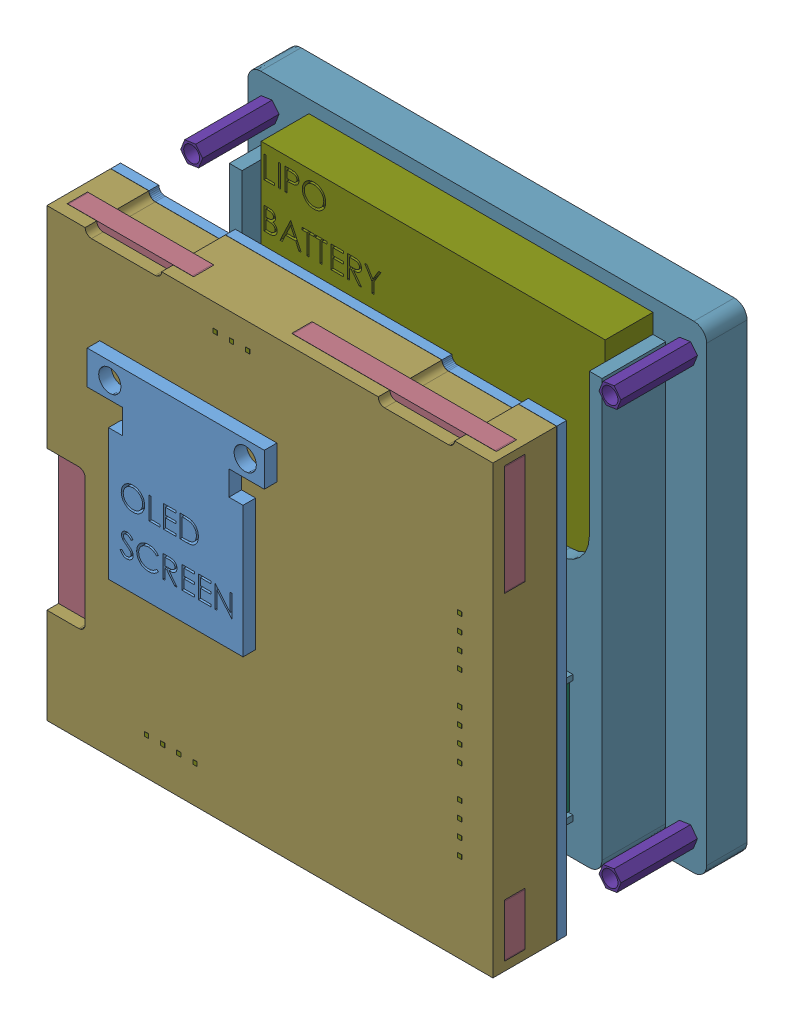
SolidWorks assembly IoTracking_PCB_Mech, configuration Default. Lengths in mm.
Overall size (72 75 40.86).
670 component instances, 221 part files, 34 mates.
Components (placement in the parent):
- IoTracking_PCBboard-1: IoTracking_PCBboard [Default] at origin size (70 70 13.59)
  - IoTracking_PCB_new.step-1: IoTracking_PCB_new.step [Default] at origin size (70.02 70.02 13.59)
    - Board.step-1: Board.step [Default] at origin size (70 70 1.53)
      - Open CASCADE STEP translator 6.8 1.1.1.step-1: Open CASCADE STEP translator 6.8 1.1.1.step [Default] at (0 0 -1.5342) size (70 70 1.53)
    - TP8.step-1: TP8.step [Default] at origin size (1.27 1.27 0.02)
      - 6125959248.step-1: 6125959248.step [Default] at (42.672 22.86 -0.015) x (-1 0 0) z (0 0 1) size (1.27 1.27 0.02)
        - Cylinder.step-1: Cylinder.step [Default] at origin size (1.27 1.27 0.02)
    - C3.step-1: C3.step [Default] at origin size (0.95 1.75 0.95)
      - 6125953728.step-1: 6125953728.step [Default] at (3.302 59.817 0) size (0.95 0.95 0.95)
        - Extruded.step-1: Extruded.step [Default] at origin size (0.95 0.95 0.95)
      - 6125953568.step-1: 6125953568.step [Default] at (3.302 59.142 0) size (0.95 0.4 0.95)
        - Extruded-0.step-1: Extruded-0.step [Default] at origin size (0.95 0.4 0.95)
      - 6125953568.step-2: 6125953568.step [Default] at (3.302 60.492 0) size (0.95 0.4 0.95)
        - Extruded-0.step-1: Extruded-0.step [Default] at origin size (0.95 0.4 0.95)
    - B1.step-1: B1.step [Default] at origin size (4.6 3.2 2.5)
      - PTS810_CK_Switch.step-1: PTS810_CK_Switch.step [Default] at (30.9881 5.5881 0) x (1 0 0) z (0 -1 0) size (4.6 2.5 3.2)
    - C9.step-1: C9.step [Default] at origin size (2.01 1.25 1.52)
      - Cap_AVX_0805YA103FAT2A_eec.step-1: Cap_AVX_0805YA103FAT2A_eec.step [Default] at (32.512 16.764 0) x (1 0 0) z (0 0 1) size (2.01 1.25 1.52)
        - Terminals.step-1: Terminals.step [Default] at origin size (2.01 1.25 1.52)
        - Electrode.step-1: Electrode.step [Default] at origin size (1.01 1.25 1.52)
        - AVX.step-1: AVX.step [Default] at origin size (0.37 0.13 0)
    - X1.step-1: X1.step [Default] at origin size (1.5 3.2 0.9)
      - 6125955888.step-1: 6125955888.step [Default] at (39.37 30.48 0) size (1.5 3.2 0.9)
        - Extruded-1.step-1: Extruded-1.step [Default] at origin size (1.5 3.2 0.9)
    - U_Buck1.step-1: U_Buck1.step [Default] at origin size (2 2 0.8)
      - 5928732880.step-1: 5928732880.step [Default] at (42.418 45.466 0) x (0 1 0) z (1 0 0) size (2 0.8 2)
    - U_Accel1.step-1: U_Accel1.step [Default] at origin size (2.5 3 1)
      - 6125958608.step-1: 6125958608.step [Default] at (21.1836 40.64 0) size (2.5 3 1)
        - Extruded-2.step-1: Extruded-2.step [Default] at origin size (2.5 3 1)
    - U4.step-1: U4.step [Default] at origin size (3.15 3.15 1)
      - 6127423232.step-1: 6127423232.step [Default] at (29.464 55.88 0) size (3.15 3.15 1)
        - Extruded-3.step-1: Extruded-3.step [Default] at origin size (3.15 3.15 1)
    - U3.step-1: U3.step [Default] at origin size (33.86 14.91 3.4)
      - SAMW25.step-1: SAMW25.step [Default] at (60.2291 61.0334 0) x (1 0 0) z (0 0 1) size (33.86 14.91 3.4)
        - wifimodule.step-1: wifimodule.step [Default] at (-37.621 -27.6339 0) x (-1 0 0) z (0 0 1) size (26.34 13.71 2.64)
        - wifimodule_2.step-1: wifimodule_2.step [Default] at (-37.621 -27.6339 0) x (-1 0 0) z (0 0 1) size (0.33 0.95 0.33)
        - wifimodule_3.step-1: wifimodule_3.step [Default] at (-37.621 -27.6339 0) x (-1 0 0) z (0 0 1) size (0.95 0.33 0.33)
        - wifimodule_4.step-1: wifimodule_4.step [Default] at (-37.621 -27.6339 0) x (-1 0 0) z (0 0 1) size (0.33 0.95 0.33)
        - wifimodule_5.step-1: wifimodule_5.step [Default] at (-37.621 -27.6339 0) x (-1 0 0) z (0 0 1) size (0.33 0.95 0.33)
        - wifimodule_6.step-1: wifimodule_6.step [Default] at (-37.621 -27.6339 0) x (-1 0 0) z (0 0 1) size (0.33 0.95 0.33)
        - wifimodule_7.step-1: wifimodule_7.step [Default] at (-37.621 -27.6339 0) x (-1 0 0) z (0 0 1) size (3.7 2.1 0.6)
        - wifimodule_8.step-1: wifimodule_8.step [Default] at (-37.621 -27.6339 0) x (-1 0 0) z (0 0 1) size (0.33 0.95 0.33)
        - wifimodule_9.step-1: wifimodule_9.step [Default] at (-37.621 -27.6339 0) x (-1 0 0) z (0 0 1) size (0.5 1 0.03)
        - wifimodule_10.step-1: wifimodule_10.step [Default] at (-37.621 -27.6339 0) x (-1 0 0) z (0 0 1) size (0.5 1 0.03)
        - wifimodule_11.step-1: wifimodule_11.step [Default] at (-37.621 -27.6339 0) x (-1 0 0) z (0 0 1) size (0.5 1 0.03)
        - wifimodule_12.step-1: wifimodule_12.step [Default] at (-37.621 -27.6339 0) x (-1 0 0) z (0 0 1) size (0.5 1 0.03)
        - wifimodule_13.step-1: wifimodule_13.step [Default] at (-37.621 -27.6339 0) x (-1 0 0) z (0 0 1) size (0.5 1 0.03)
        - wifimodule_14.step-1: wifimodule_14.step [Default] at (-37.621 -27.6339 0) x (-1 0 0) z (0 0 1) size (0.5 1 0.03)
        - wifimodule_15.step-1: wifimodule_15.step [Default] at (-37.621 -27.6339 0) x (-1 0 0) z (0 0 1) size (0.5 1 0.03)
        - wifimodule_16.step-1: wifimodule_16.step [Default] at (-37.621 -27.6339 0) x (-1 0 0) z (0 0 1) size (0.5 1 0.03)
        - wifimodule_17.step-1: wifimodule_17.step [Default] at (-37.621 -27.6339 0) x (-1 0 0) z (0 0 1) size (0.5 1 0.03)
        - wifimodule_18.step-1: wifimodule_18.step [Default] at (-37.621 -27.6339 0) x (-1 0 0) z (0 0 1) size (0.5 1 0.03)
        - wifimodule_19.step-1: wifimodule_19.step [Default] at (-37.621 -27.6339 0) x (-1 0 0) z (0 0 1) size (0.5 1 0.03)
        - wifimodule_20.step-1: wifimodule_20.step [Default] at (-37.621 -27.6339 0) x (-1 0 0) z (0 0 1) size (0.5 1 0.03)
        - wifimodule_21.step-1: wifimodule_21.step [Default] at (-37.621 -27.6339 0) x (-1 0 0) z (0 0 1) size (0.5 1 0.03)
        - wifimodule_22.step-1: wifimodule_22.step [Default] at (-37.621 -27.6339 0) x (-1 0 0) z (0 0 1) size (0.5 1 0.03)
        - wifimodule_23.step-1: wifimodule_23.step [Default] at (-37.621 -27.6339 0) x (-1 0 0) z (0 0 1) size (0.5 1 0.03)
        - wifimodule_24.step-1: wifimodule_24.step [Default] at (-37.621 -27.6339 0) x (-1 0 0) z (0 0 1) size (0.95 0.33 0.33)
        - wifimodule_25.step-1: wifimodule_25.step [Default] at (-37.621 -27.6339 0) x (-1 0 0) z (0 0 1) size (0.95 0.33 0.33)
        - wifimodule_26.step-1: wifimodule_26.step [Default] at (-37.621 -27.6339 0) x (-1 0 0) z (0 0 1) size (0.95 0.33 0.33)
        - wifimodule_27.step-1: wifimodule_27.step [Default] at (-37.621 -27.6339 0) x (-1 0 0) z (0 0 1) size (0.33 0.95 0.33)
        - wifimodule_28.step-1: wifimodule_28.step [Default] at (-37.621 -27.6339 0) x (-1 0 0) z (0 0 1) size (0.95 0.33 0.33)
        - wifimodule_29.step-1: wifimodule_29.step [Default] at (-37.621 -27.6339 0) x (-1 0 0) z (0 0 1) size (0.33 0.95 0.33)
        - wifimodule_30.step-1: wifimodule_30.step [Default] at (-37.621 -27.6339 0) x (-1 0 0) z (0 0 1) size (0.95 0.33 0.33)
        - wifimodule_31.step-1: wifimodule_31.step [Default] at (-37.621 -27.6339 0) x (-1 0 0) z (0 0 1) size (0.33 0.95 0.33)
        - wifimodule_32.step-1: wifimodule_32.step [Default] at (-37.621 -27.6339 0) x (-1 0 0) z (0 0 1) size (0.33 0.74 1)
        - wifimodule_33.step-1: wifimodule_33.step [Default] at (-37.621 -27.6339 0) x (-1 0 0) z (0 0 1) size (0.74 0.33 1)
        - wifimodule_34.step-1: wifimodule_34.step [Default] at (-37.621 -27.6339 0) x (-1 0 0) z (0 0 1) size (2.68 1.78 1.04)
        - wifimodule_35.step-1: wifimodule_35.step [Default] at (-37.621 -27.6339 0) x (-1 0 0) z (0 0 1) size (1.56 1.02 0.66)
        - wifimodule_36.step-1: wifimodule_36.step [Default] at (-37.621 -27.6339 0) x (-1 0 0) z (0 0 1) size (0.91 2.06 0.41)
        - wifimodule_37.step-1: wifimodule_37.step [Default] at (-37.621 -27.6339 0) x (-1 0 0) z (0 0 1) size (2.06 0.91 0.41)
        - wifimodule_38.step-1: wifimodule_38.step [Default] at (-37.621 -27.6339 0) x (-1 0 0) z (0 0 1) size (2.06 0.91 0.41)
        - wifimodule_39.step-1: wifimodule_39.step [Default] at (-37.621 -27.6339 0) x (-1 0 0) z (0 0 1) size (0.91 2.06 0.41)
        - wifimodule_40.step-1: wifimodule_40.step [Default] at (-37.621 -27.6339 0) x (-1 0 0) z (0 0 1) size (0.33 0.74 1)
        - wifimodule_41.step-1: wifimodule_41.step [Default] at (-37.621 -27.6339 0) x (-1 0 0) z (0 0 1) size (0.33 0.74 1)
        - wifimodule_42.step-1: wifimodule_42.step [Default] at (-37.621 -27.6339 0) x (-1 0 0) z (0 0 1) size (0.33 0.74 1)
        - wifimodule_43.step-1: wifimodule_43.step [Default] at (-37.621 -27.6339 0) x (-1 0 0) z (0 0 1) size (0.33 0.74 1)
        - wifimodule_44.step-1: wifimodule_44.step [Default] at (-37.621 -27.6339 0) x (-1 0 0) z (0 0 1) size (0.33 0.74 1)
        - wifimodule_45.step-1: wifimodule_45.step [Default] at (-37.621 -27.6339 0) x (-1 0 0) z (0 0 1) size (0.74 0.33 1)
        - wifimodule_46.step-1: wifimodule_46.step [Default] at (-37.621 -27.6339 0) x (-1 0 0) z (0 0 1) size (0.74 0.33 1)
        - wifimodule_47.step-1: wifimodule_47.step [Default] at (-37.621 -27.6339 0) x (-1 0 0) z (0 0 1) size (0.33 0.74 1)
        - wifimodule_48.step-1: wifimodule_48.step [Default] at (-37.621 -27.6339 0) x (-1 0 0) z (0 0 1) size (0.33 0.74 1)
        - wifimodule_49.step-1: wifimodule_49.step [Default] at (-37.621 -27.6339 0) x (-1 0 0) z (0 0 1) size (0.33 0.74 1)
        - wifimodule_50.step-1: wifimodule_50.step [Default] at (-37.621 -27.6339 0) x (-1 0 0) z (0 0 1) size (0.74 0.33 1)
        - wifimodule_51.step-1: wifimodule_51.step [Default] at (-37.621 -27.6339 0) x (-1 0 0) z (0 0 1) size (0.74 0.33 1)
        - wifimodule_52.step-1: wifimodule_52.step [Default] at (-37.621 -27.6339 0) x (-1 0 0) z (0 0 1) size (0.74 0.33 1)
        - wifimodule_53.step-1: wifimodule_53.step [Default] at (-37.621 -27.6339 0) x (-1 0 0) z (0 0 1) size (0.74 0.33 1)
        - wifimodule_54.step-1: wifimodule_54.step [Default] at (-37.621 -27.6339 0) x (-1 0 0) z (0 0 1) size (0.74 0.33 1)
        - wifimodule_55.step-1: wifimodule_55.step [Default] at (-37.621 -27.6339 0) x (-1 0 0) z (0 0 1) size (0.33 0.74 1)
        - wifimodule_56.step-1: wifimodule_56.step [Default] at (-37.621 -27.6339 0) x (-1 0 0) z (0 0 1) size (0.74 0.33 1)
        - wifimodule_57.step-1: wifimodule_57.step [Default] at (-37.621 -27.6339 0) x (-1 0 0) z (0 0 1) size (0.42 1.12 0.33)
        - wifimodule_58.step-1: wifimodule_58.step [Default] at (-37.621 -27.6339 0) x (-1 0 0) z (0 0 1) size (0.5 1 0.03)
        - wifimodule_59.step-1: wifimodule_59.step [Default] at (-37.621 -27.6339 0) x (-1 0 0) z (0 0 1) size (0.42 1.12 0.33)
        - wifimodule_60.step-1: wifimodule_60.step [Default] at (-37.621 -27.6339 0) x (-1 0 0) z (0 0 1) size (3.66 4.34 0.91)
        - wifimodule_61.step-1: wifimodule_61.step [Default] at (-37.621 -27.6339 0) x (-1 0 0) z (0 0 1) size (0.5 1 0.03)
        - wifimodule_62.step-1: wifimodule_62.step [Default] at (-37.621 -27.6339 0) x (-1 0 0) z (0 0 1) size (0.5 1 0.03)
        - wifimodule_63.step-1: wifimodule_63.step [Default] at (-37.621 -27.6339 0) x (-1 0 0) z (0 0 1) size (0.5 1 0.03)
        - wifimodule_64.step-1: wifimodule_64.step [Default] at (-37.621 -27.6339 0) x (-1 0 0) z (0 0 1) size (0.5 1 0.03)
        - wifimodule_65.step-1: wifimodule_65.step [Default] at (-37.621 -27.6339 0) x (-1 0 0) z (0 0 1) size (1 0.5 0.03)
        - wifimodule_66.step-1: wifimodule_66.step [Default] at (-37.621 -27.6339 0) x (-1 0 0) z (0 0 1) size (1 0.5 0.03)
        - wifimodule_67.step-1: wifimodule_67.step [Default] at (-37.621 -27.6339 0) x (-1 0 0) z (0 0 1) size (1 0.5 0.03)
        - wifimodule_68.step-1: wifimodule_68.step [Default] at (-37.621 -27.6339 0) x (-1 0 0) z (0 0 1) size (1 0.5 0.03)
        - wifimodule_69.step-1: wifimodule_69.step [Default] at (-37.621 -27.6339 0) x (-1 0 0) z (0 0 1) size (1 0.5 0.03)
        - wifimodule_70.step-1: wifimodule_70.step [Default] at (-37.621 -27.6339 0) x (-1 0 0) z (0 0 1) size (1 0.5 0.03)
        - wifimodule_71.step-1: wifimodule_71.step [Default] at (-37.621 -27.6339 0) x (-1 0 0) z (0 0 1) size (1 0.5 0.03)
        - wifimodule_72.step-1: wifimodule_72.step [Default] at (-37.621 -27.6339 0) x (-1 0 0) z (0 0 1) size (0.5 1 0.03)
        - wifimodule_73.step-1: wifimodule_73.step [Default] at (-37.621 -27.6339 0) x (-1 0 0) z (0 0 1) size (0.5 1 0.03)
        - wifimodule_74.step-1: wifimodule_74.step [Default] at (-37.621 -27.6339 0) x (-1 0 0) z (0 0 1) size (0.5 1 0.03)
        - wifimodule_75.step-1: wifimodule_75.step [Default] at (-37.621 -27.6339 0) x (-1 0 0) z (0 0 1) size (0.5 1 0.03)
        - wifimodule_76.step-1: wifimodule_76.step [Default] at (-37.621 -27.6339 0) x (-1 0 0) z (0 0 1) size (0.5 1 0.03)
        - wifimodule_77.step-1: wifimodule_77.step [Default] at (-37.621 -27.6339 0) x (-1 0 0) z (0 0 1) size (0.5 1 0.03)
        - wifimodule_78.step-1: wifimodule_78.step [Default] at (-37.621 -27.6339 0) x (-1 0 0) z (0 0 1) size (0.5 1 0.03)
        - wifimodule_79.step-1: wifimodule_79.step [Default] at (-37.621 -27.6339 0) x (-1 0 0) z (0 0 1) size (0.5 1 0.03)
        - wifimodule_80.step-1: wifimodule_80.step [Default] at (-37.621 -27.6339 0) x (-1 0 0) z (0 0 1) size (0.95 0.33 0.33)
        - wifimodule_81.step-1: wifimodule_81.step [Default] at (-37.621 -27.6339 0) x (-1 0 0) z (0 0 1) size (0.95 0.33 0.33)
        - wifimodule_82.step-1: wifimodule_82.step [Default] at (-37.621 -27.6339 0) x (-1 0 0) z (0 0 1) size (0.33 0.95 0.33)
        - wifimodule_83.step-1: wifimodule_83.step [Default] at (-37.621 -27.6339 0) x (-1 0 0) z (0 0 1) size (0.33 0.95 0.33)
        - wifimodule_84.step-1: wifimodule_84.step [Default] at (-37.621 -27.6339 0) x (-1 0 0) z (0 0 1) size (1.12 0.42 0.33)
        - wifimodule_85.step-1: wifimodule_85.step [Default] at (-37.621 -27.6339 0) x (-1 0 0) z (0 0 1) size (0.95 0.33 0.33)
        - wifimodule_86.step-1: wifimodule_86.step [Default] at (-37.621 -27.6339 0) x (-1 0 0) z (0 0 1) size (0.42 1.12 0.33)
        - wifimodule_87.step-1: wifimodule_87.step [Default] at (-37.621 -27.6339 0) x (-1 0 0) z (0 0 1) size (0.95 0.33 0.33)
        - wifimodule_88.step-1: wifimodule_88.step [Default] at (-37.621 -27.6339 0) x (-1 0 0) z (0 0 1) size (1 0.5 0.03)
        - wifimodule_89.step-1: wifimodule_89.step [Default] at (-37.621 -27.6339 0) x (-1 0 0) z (0 0 1) size (0.5 1 0.03)
        - wifimodule_90.step-1: wifimodule_90.step [Default] at (-37.621 -27.6339 0) x (-1 0 0) z (0 0 1) size (0.5 1 0.03)
        - wifimodule_91.step-1: wifimodule_91.step [Default] at (-37.621 -27.6339 0) x (-1 0 0) z (0 0 1) size (0.5 1 0.03)
        - wifimodule_92.step-1: wifimodule_92.step [Default] at (-37.621 -27.6339 0) x (-1 0 0) z (0 0 1) size (1 0.5 0.03)
        - wifimodule_93.step-1: wifimodule_93.step [Default] at (-37.621 -27.6339 0) x (-1 0 0) z (0 0 1) size (0.5 1 0.03)
        - wifimodule_94.step-1: wifimodule_94.step [Default] at (-37.621 -27.6339 0) x (-1 0 0) z (0 0 1) size (0.5 1 0.03)
        - wifimodule_95.step-1: wifimodule_95.step [Default] at (-37.621 -27.6339 0) x (-1 0 0) z (0 0 1) size (0.5 1 0.03)
        - wifimodule_96.step-1: wifimodule_96.step [Default] at (-37.621 -27.6339 0) x (-1 0 0) z (0 0 1) size (0.5 1 0.03)
        - wifimodule_97.step-1: wifimodule_97.step [Default] at (-37.621 -27.6339 0) x (-1 0 0) z (0 0 1) size (0.5 1 0.03)
        - wifimodule_98.step-1: wifimodule_98.step [Default] at (-37.621 -27.6339 0) x (-1 0 0) z (0 0 1) size (1 0.5 0.03)
        - wifimodule_99.step-1: wifimodule_99.step [Default] at (-37.621 -27.6339 0) x (-1 0 0) z (0 0 1) size (1 0.5 0.03)
        - wifimodule_100.step-1: wifimodule_100.step [Default] at (-37.621 -27.6339 0) x (-1 0 0) z (0 0 1) size (0.5 1 0.03)
        - wifimodule_101.step-1: wifimodule_101.step [Default] at (-37.621 -27.6339 0) x (-1 0 0) z (0 0 1) size (0.5 1 0.03)
        - wifimodule_102.step-1: wifimodule_102.step [Default] at (-37.621 -27.6339 0) x (-1 0 0) z (0 0 1) size (0.5 1 0.03)
        - wifimodule_103.step-1: wifimodule_103.step [Default] at (-37.621 -27.6339 0) x (-1 0 0) z (0 0 1) size (0.5 1 0.03)
        - wifimodule_104.step-1: wifimodule_104.step [Default] at (-37.621 -27.6339 0) x (-1 0 0) z (0 0 1) size (0.33 0.95 0.33)
        - wifimodule_105.step-1: wifimodule_105.step [Default] at (-37.621 -27.6339 0) x (-1 0 0) z (0 0 1) size (0.33 0.95 0.33)
        - wifimodule_106.step-1: wifimodule_106.step [Default] at (-37.621 -27.6339 0) x (-1 0 0) z (0 0 1) size (0.33 0.95 0.33)
        - wifimodule_107.step-1: wifimodule_107.step [Default] at (-37.621 -27.6339 0) x (-1 0 0) z (0 0 1) size (0.33 0.95 0.33)
        - wifimodule_108.step-1: wifimodule_108.step [Default] at (-37.621 -27.6339 0) x (-1 0 0) z (0 0 1) size (0.95 0.33 0.33)
        - wifimodule_109.step-1: wifimodule_109.step [Default] at (-37.621 -27.6339 0) x (-1 0 0) z (0 0 1) size (0.33 0.95 0.33)
        - wifimodule_110.step-1: wifimodule_110.step [Default] at (-37.621 -27.6339 0) x (-1 0 0) z (0 0 1) size (0.33 0.95 0.33)
        - wifimodule_111.step-1: wifimodule_111.step [Default] at (-37.621 -27.6339 0) x (-1 0 0) z (0 0 1) size (0.74 0.33 1)
        - wifimodule_112.step-1: wifimodule_112.step [Default] at (-37.621 -27.6339 0) x (-1 0 0) z (0 0 1) size (0.91 2.06 0.41)
        - wifimodule_113.step-1: wifimodule_113.step [Default] at (-37.621 -27.6339 0) x (-1 0 0) z (0 0 1) size (0.89 0.89 0.03)
        - wifimodule_114.step-1: wifimodule_114.step [Default] at (-37.621 -27.6339 0) x (-1 0 0) z (0 0 1) size (5.4 14.4 0.03)
        - wifimodule_115.step-1: wifimodule_115.step [Default] at (-37.621 -27.6339 0) x (-1 0 0) z (0 0 1) size (33.86 14.91 0.73)
        - wifimodule_116.step-1: wifimodule_116.step [Default] at (-37.621 -27.6339 0) x (-1 0 0) z (0 0 1) size (2.5 2.2 1.1)
        - wifimodule_117.step-1: wifimodule_117.step [Default] at (-37.621 -27.6339 0) x (-1 0 0) z (0 0 1) size (7.2 7.2 0.9)
        - wifimodule_118.step-1: wifimodule_118.step [Default] at (-37.621 -27.6339 0) x (-1 0 0) z (0 0 1) size (5.6 5.6 0.85)
    - U2.step-1: U2.step [Default] at origin size (3.4 6.35 7.85)
      - 10posheader.step-1: 10posheader.step [Default] at (38.989 22.86 0) x (0 -1 0) z (-1 0 0) size (6.35 7.85 3.4)
    - U1.step-1: U1.step [Default] at origin size (3 3 0.9)
      - 6127410672.step-1: 6127410672.step [Default] at (13.8684 51.7906 0) size (3 3 0.9)
        - Extruded-4.step-1: Extruded-4.step [Default] at origin size (3 3 0.9)
    - TP_OLED_2.step-1: TP_OLED_2.step [Default] at origin size (1.27 1.27 0.02)
      - 6127428272.step-1: 6127428272.step [Default] at (9.906 8.128 -0.015) x (0 1 0) z (0 0 1) size (1.27 1.27 0.02)
        - Cylinder-5.step-1: Cylinder-5.step [Default] at origin size (1.27 1.27 0.02)
    - TP_OLED_1.step-1: TP_OLED_1.step [Default] at origin size (1.27 1.27 0.02)
      - 6127428272.step-1: 6127428272.step [Default] at (9.906 3.556 -0.015) x (0 1 0) z (0 0 1) size (1.27 1.27 0.02)
        - Cylinder-5.step-1: Cylinder-5.step [Default] at origin size (1.27 1.27 0.02)
    - TP_GPS_2.step-1: TP_GPS_2.step [Default] at origin size (1.27 1.27 0.02)
      - 6127428272.step-1: 6127428272.step [Default] at (49.53 34.29 -0.015) x (0 1 0) z (0 0 1) size (1.27 1.27 0.02)
        - Cylinder-5.step-1: Cylinder-5.step [Default] at origin size (1.27 1.27 0.02)
    - TP_GPS_1.step-1: TP_GPS_1.step [Default] at origin size (1.27 1.27 0.02)
      - 6127428272.step-1: 6127428272.step [Default] at (49.53 31.75 -0.015) x (0 1 0) z (0 0 1) size (1.27 1.27 0.02)
        - Cylinder-5.step-1: Cylinder-5.step [Default] at origin size (1.27 1.27 0.02)
    - TP_BUCK_2.step-1: TP_BUCK_2.step [Default] at origin size (1.27 1.27 0.02)
      - 6127428272.step-1: 6127428272.step [Default] at (41.275 40.005 -0.015) x (0 1 0) z (0 0 1) size (1.27 1.27 0.02)
        - Cylinder-5.step-1: Cylinder-5.step [Default] at origin size (1.27 1.27 0.02)
    - TP_BUCK_1.step-1: TP_BUCK_1.step [Default] at origin size (1.27 1.27 0.02)
      - 6126688688.step-1: 6126688688.step [Default] at (45.7962 39.751 -0.015) x (1 0 0) z (0 0 1) size (1.27 1.27 0.02)
        - Cylinder-6.step-1: Cylinder-6.step [Default] at origin size (1.27 1.27 0.02)
    - TP_ACC_2.step-1: TP_ACC_2.step [Default] at origin size (1.27 1.27 0.02)
      - 6127428272.step-1: 6127428272.step [Default] at (30.48 43.815 -0.015) x (0 1 0) z (0 0 1) size (1.27 1.27 0.02)
        - Cylinder-5.step-1: Cylinder-5.step [Default] at origin size (1.27 1.27 0.02)
    - TP_ACC_1.step-1: TP_ACC_1.step [Default] at origin size (1.27 1.27 0.02)
      - 6127428272.step-1: 6127428272.step [Default] at (30.48 38.1762 -0.015) x (0 1 0) z (0 0 1) size (1.27 1.27 0.02)
        - Cylinder-5.step-1: Cylinder-5.step [Default] at origin size (1.27 1.27 0.02)
    - TP16.step-1: TP16.step [Default] at origin size (1.27 1.27 0.02)
      - 6125959248.step-1: 6125959248.step [Default] at (45.974 59.944 -0.015) x (-1 0 0) z (0 0 1) size (1.27 1.27 0.02)
        - Cylinder.step-1: Cylinder.step [Default] at origin size (1.27 1.27 0.02)
    - TP15.step-1: TP15.step [Default] at origin size (1.27 1.27 0.02)
      - 6125959248.step-1: 6125959248.step [Default] at (61.595 55.118 -0.015) x (-1 0 0) z (0 0 1) size (1.27 1.27 0.02)
        - Cylinder.step-1: Cylinder.step [Default] at origin size (1.27 1.27 0.02)
    - TP14.step-1: TP14.step [Default] at origin size (1.27 1.27 0.02)
      - 6125959248.step-1: 6125959248.step [Default] at (65.786 55.118 -0.015) x (-1 0 0) z (0 0 1) size (1.27 1.27 0.02)
        - Cylinder.step-1: Cylinder.step [Default] at origin size (1.27 1.27 0.02)
    - TP13.step-1: TP13.step [Default] at origin size (1.27 1.27 0.02)
      - 6125959248.step-1: 6125959248.step [Default] at (55.499 55.245 -0.015) x (-1 0 0) z (0 0 1) size (1.27 1.27 0.02)
        - Cylinder.step-1: Cylinder.step [Default] at origin size (1.27 1.27 0.02)
    - TP12.step-1: TP12.step [Default] at origin size (1.27 1.27 0.02)
      - 6127428272.step-1: 6127428272.step [Default] at (49.911 59.944 -0.015) x (0 1 0) z (0 0 1) size (1.27 1.27 0.02)
        - Cylinder-5.step-1: Cylinder-5.step [Default] at origin size (1.27 1.27 0.02)
    - TP11.step-1: TP11.step [Default] at origin size (1.27 1.27 0.02)
      - 6127428272.step-1: 6127428272.step [Default] at (45.974 64.008 -0.015) x (0 1 0) z (0 0 1) size (1.27 1.27 0.02)
        - Cylinder-5.step-1: Cylinder-5.step [Default] at origin size (1.27 1.27 0.02)
    - TP10.step-1: TP10.step [Default] at origin size (1.27 1.27 0.02)
      - 6125959248.step-1: 6125959248.step [Default] at (44.958 19.05 -0.015) x (-1 0 0) z (0 0 1) size (1.27 1.27 0.02)
        - Cylinder.step-1: Cylinder.step [Default] at origin size (1.27 1.27 0.02)
    - TP9.step-1: TP9.step [Default] at origin size (1.27 1.27 0.02)
      - 6125959248.step-1: 6125959248.step [Default] at (44.958 21.59 -0.015) x (-1 0 0) z (0 0 1) size (1.27 1.27 0.02)
        - Cylinder.step-1: Cylinder.step [Default] at origin size (1.27 1.27 0.02)
    - TP7.step-1: TP7.step [Default] at origin size (1.27 1.27 0.02)
      - 6125959248.step-1: 6125959248.step [Default] at (42.672 20.32 -0.015) x (-1 0 0) z (0 0 1) size (1.27 1.27 0.02)
        - Cylinder.step-1: Cylinder.step [Default] at origin size (1.27 1.27 0.02)
    - TP6.step-1: TP6.step [Default] at origin size (1.27 1.27 0.02)
      - 6125959248.step-1: 6125959248.step [Default] at (44.958 24.13 -0.015) x (-1 0 0) z (0 0 1) size (1.27 1.27 0.02)
        - Cylinder.step-1: Cylinder.step [Default] at origin size (1.27 1.27 0.02)
    - TP5.step-1: TP5.step [Default] at origin size (1.27 1.27 0.02)
      - 6127428272.step-1: 6127428272.step [Default] at (35.56 59.8932 -0.015) x (0 1 0) z (0 0 1) size (1.27 1.27 0.02)
        - Cylinder-5.step-1: Cylinder-5.step [Default] at origin size (1.27 1.27 0.02)
    - TP4.step-1: TP4.step [Default] at origin size (1.27 1.27 0.02)
      - 6127428272.step-1: 6127428272.step [Default] at (14.224 40.8444 -0.015) x (0 1 0) z (0 0 1) size (1.27 1.27 0.02)
        - Cylinder-5.step-1: Cylinder-5.step [Default] at origin size (1.27 1.27 0.02)
    - TP3.step-1: TP3.step [Default] at origin size (1.27 1.27 0.02)
      - 6127428272.step-1: 6127428272.step [Default] at (19.8882 16.51 -0.015) x (0 1 0) z (0 0 1) size (1.27 1.27 0.02)
        - Cylinder-5.step-1: Cylinder-5.step [Default] at origin size (1.27 1.27 0.02)
    - TP2.step-1: TP2.step [Default] at origin size (1.27 1.27 0.02)
      - 6127428272.step-1: 6127428272.step [Default] at (15.8242 40.8686 -0.015) x (0 1 0) z (0 0 1) size (1.27 1.27 0.02)
        - Cylinder-5.step-1: Cylinder-5.step [Default] at origin size (1.27 1.27 0.02)
    - TP1.step-1: TP1.step [Default] at origin size (1.27 1.27 0.02)
      - 6127428272.step-1: 6127428272.step [Default] at (20.066 65.024 -0.015) x (0 1 0) z (0 0 1) size (1.27 1.27 0.02)
        - Cylinder-5.step-1: Cylinder-5.step [Default] at origin size (1.27 1.27 0.02)
    - SD1.step-1: SD1.step [Default] at origin size (11.95 11.4 1.45)
      - 1040310811.step-1: 1040310811.step [Default] at (102.3746 60.988 0.61) x (-1 0 0) z (0 0 1) size (11.95 11.4 1.45)
        - Open CASCADE STEP translator 6.8 1.36.1.1.step-1: Open CASCADE STEP translator 6.8 1.36.1.1.step [Default] at origin size (11.95 11.4 1.45)
        - Open CASCADE STEP translator 6.8 1.36.1.2.step-1: Open CASCADE STEP translator 6.8 1.36.1.2.step [Default] at origin
    - RJ1.step-1: RJ1.step [Default] at origin size (1.65 0.95 0.5)
      - 6125952048.step-1: 6125952048.step [Default] at (38.354 41.656 0) size (1.05 0.95 0.5)
        - Extruded-7.step-1: Extruded-7.step [Default] at origin size (1.05 0.95 0.5)
      - 6125951888.step-1: 6125951888.step [Default] at (37.679 41.656 0) size (0.3 0.95 0.5)
        - Extruded-8.step-1: Extruded-8.step [Default] at origin size (0.3 0.95 0.5)
      - 6125951888.step-2: 6125951888.step [Default] at (39.029 41.656 0) size (0.3 0.95 0.5)
        - Extruded-8.step-1: Extruded-8.step [Default] at origin size (0.3 0.95 0.5)
    - R_O2.step-1: R_O2.step [Default] at origin size (1.6 0.8 0.55)
      - Res_Yageo_AT0603CRD0711R5L_eec.step-1: Res_Yageo_AT0603CRD0711R5L_eec.step [Default] at (19.05 10.414 0) x (-1 0 0) z (0 0 1) size (1.6 0.8 0.55)
        - 2.step-1: 2.step [Default] at origin size (1.6 0.8 0.55)
          - Open CASCADE STEP translator 6.8 1.38.1.1.1.step-1: Open CASCADE STEP translator 6.8 1.38.1.1.1.step [Default] at origin size (1.6 0.8 0.55)
          - Open CASCADE STEP translator 6.8 1.38.1.1.2.step-1: Open CASCADE STEP translator 6.8 1.38.1.1.2.step [Default] at origin
        - 3.step-1: 3.step [Default] at origin size (1.5 0.8 0.45)
          - Open CASCADE STEP translator 6.8 1.38.1.2.1.step-1: Open CASCADE STEP translator 6.8 1.38.1.2.1.step [Default] at origin size (1.5 0.8 0.45)
          - Open CASCADE STEP translator 6.8 1.38.1.2.2.step-1: Open CASCADE STEP translator 6.8 1.38.1.2.2.step [Default] at origin
        - 4.step-1: 4.step [Default] at origin size (1.2 0.8 0.05)
          - Open CASCADE STEP translator 6.8 1.38.1.3.1.step-1: Open CASCADE STEP translator 6.8 1.38.1.3.1.step [Default] at origin size (1.2 0.8 0.05)
          - Open CASCADE STEP translator 6.8 1.38.1.3.2.step-1: Open CASCADE STEP translator 6.8 1.38.1.3.2.step [Default] at origin
        - 5.step-1: 5.step [Default] at (-0.0114 0.0028 0.4505) size (0.29 0.05 0.11)
    - R_O1.step-1: R_O1.step [Default] at origin size (1.6 0.8 0.55)
      - Res_Yageo_AT0603CRD0711R5L_eec.step-1: Res_Yageo_AT0603CRD0711R5L_eec.step [Default] at (14.732 10.414 0) x (1 0 0) z (0 0 1) size (1.6 0.8 0.55)
        - 2.step-1: 2.step [Default] at origin size (1.6 0.8 0.55)
          - Open CASCADE STEP translator 6.8 1.38.1.1.1.step-1: Open CASCADE STEP translator 6.8 1.38.1.1.1.step [Default] at origin size (1.6 0.8 0.55)
          - Open CASCADE STEP translator 6.8 1.38.1.1.2.step-1: Open CASCADE STEP translator 6.8 1.38.1.1.2.step [Default] at origin
        - 3.step-1: 3.step [Default] at origin size (1.5 0.8 0.45)
          - Open CASCADE STEP translator 6.8 1.38.1.2.1.step-1: Open CASCADE STEP translator 6.8 1.38.1.2.1.step [Default] at origin size (1.5 0.8 0.45)
          - Open CASCADE STEP translator 6.8 1.38.1.2.2.step-1: Open CASCADE STEP translator 6.8 1.38.1.2.2.step [Default] at origin
        - 4.step-1: 4.step [Default] at origin size (1.2 0.8 0.05)
          - Open CASCADE STEP translator 6.8 1.38.1.3.1.step-1: Open CASCADE STEP translator 6.8 1.38.1.3.1.step [Default] at origin size (1.2 0.8 0.05)
          - Open CASCADE STEP translator 6.8 1.38.1.3.2.step-1: Open CASCADE STEP translator 6.8 1.38.1.3.2.step [Default] at origin
        - 5.step-1: 5.step [Default] at (-0.0114 0.0028 0.4505) size (0.29 0.05 0.11)
    - R_B1.step-1: R_B1.step [Default] at origin size (1.55 0.8 0.56)
      - Res_TE_Connectivity_CPF0603B2K55E1_eec.step-1: Res_TE_Connectivity_CPF0603B2K55E1_eec.step [Default] at (46.863 41.783 0) x (1 0 0) z (0 0 1) size (1.55 0.8 0.56)
        - 1.step-1: 1.step [Default] at origin size (1.55 0.8 0.55)
        - 2-9.step-1: 2-9.step [Default] at origin size (1.45 0.8 0.5)
        - TE_connectivity_Logo_1.step-1: TE_connectivity_Logo_1.step [Default] at (5.0457 3.7568 0.451) x (-1 0 0) z (0 0 1) size (0.47 0.17 0.11)
        - 3-10.step-1: 3-10.step [Default] at origin size (0.95 0.8 0.05)
    - R_A2.step-1: R_A2.step [Default] at origin size (0.8 1.6 0.55)
      - Res_Yageo_AT0603CRD0711R5L_eec.step-1: Res_Yageo_AT0603CRD0711R5L_eec.step [Default] at (27.686 42.926 0) x (0 -1 0) z (0 0 1) size (1.6 0.8 0.55)
        - 2.step-1: 2.step [Default] at origin size (1.6 0.8 0.55)
          - Open CASCADE STEP translator 6.8 1.38.1.1.1.step-1: Open CASCADE STEP translator 6.8 1.38.1.1.1.step [Default] at origin size (1.6 0.8 0.55)
          - Open CASCADE STEP translator 6.8 1.38.1.1.2.step-1: Open CASCADE STEP translator 6.8 1.38.1.1.2.step [Default] at origin
        - 3.step-1: 3.step [Default] at origin size (1.5 0.8 0.45)
          - Open CASCADE STEP translator 6.8 1.38.1.2.1.step-1: Open CASCADE STEP translator 6.8 1.38.1.2.1.step [Default] at origin size (1.5 0.8 0.45)
          - Open CASCADE STEP translator 6.8 1.38.1.2.2.step-1: Open CASCADE STEP translator 6.8 1.38.1.2.2.step [Default] at origin
        - 4.step-1: 4.step [Default] at origin size (1.2 0.8 0.05)
          - Open CASCADE STEP translator 6.8 1.38.1.3.1.step-1: Open CASCADE STEP translator 6.8 1.38.1.3.1.step [Default] at origin size (1.2 0.8 0.05)
          - Open CASCADE STEP translator 6.8 1.38.1.3.2.step-1: Open CASCADE STEP translator 6.8 1.38.1.3.2.step [Default] at origin
        - 5.step-1: 5.step [Default] at (-0.0114 0.0028 0.4505) size (0.29 0.05 0.11)
    - R_A1.step-1: R_A1.step [Default] at origin size (0.8 1.6 0.55)
      - Res_Yageo_AT0603CRD0711R5L_eec.step-1: Res_Yageo_AT0603CRD0711R5L_eec.step [Default] at (27.686 38.862 0) x (0 1 0) z (0 0 1) size (1.6 0.8 0.55)
        - 2.step-1: 2.step [Default] at origin size (1.6 0.8 0.55)
          - Open CASCADE STEP translator 6.8 1.38.1.1.1.step-1: Open CASCADE STEP translator 6.8 1.38.1.1.1.step [Default] at origin size (1.6 0.8 0.55)
          - Open CASCADE STEP translator 6.8 1.38.1.1.2.step-1: Open CASCADE STEP translator 6.8 1.38.1.1.2.step [Default] at origin
        - 3.step-1: 3.step [Default] at origin size (1.5 0.8 0.45)
          - Open CASCADE STEP translator 6.8 1.38.1.2.1.step-1: Open CASCADE STEP translator 6.8 1.38.1.2.1.step [Default] at origin size (1.5 0.8 0.45)
          - Open CASCADE STEP translator 6.8 1.38.1.2.2.step-1: Open CASCADE STEP translator 6.8 1.38.1.2.2.step [Default] at origin
        - 4.step-1: 4.step [Default] at origin size (1.2 0.8 0.05)
          - Open CASCADE STEP translator 6.8 1.38.1.3.1.step-1: Open CASCADE STEP translator 6.8 1.38.1.3.1.step [Default] at origin size (1.2 0.8 0.05)
          - Open CASCADE STEP translator 6.8 1.38.1.3.2.step-1: Open CASCADE STEP translator 6.8 1.38.1.3.2.step [Default] at origin
        - 5.step-1: 5.step [Default] at (-0.0114 0.0028 0.4505) size (0.29 0.05 0.11)
    - R19.step-1: R19.step [Default] at origin size (1.7 0.95 0.6)
      - 6127424752.step-1: 6127424752.step [Default] at (32.8129 56.6419 0) size (0.27 0.95 0.6)
        - Extruded-11.step-1: Extruded-11.step [Default] at origin size (0.27 0.95 0.6)
      - 6127424592.step-1: 6127424592.step [Default] at (33.5279 56.6419 0) size (1.16 0.95 0.6)
        - Extruded-12.step-1: Extruded-12.step [Default] at origin size (1.16 0.95 0.6)
      - 6127424752.step-2: 6127424752.step [Default] at (34.2429 56.6419 0) size (0.27 0.95 0.6)
        - Extruded-11.step-1: Extruded-11.step [Default] at origin size (0.27 0.95 0.6)
    - R18.step-1: R18.step [Default] at origin size (1.7 0.95 0.6)
      - 6127424752.step-1: 6127424752.step [Default] at (31.0349 51.8159 0) size (0.27 0.95 0.6)
        - Extruded-11.step-1: Extruded-11.step [Default] at origin size (0.27 0.95 0.6)
      - 6127424592.step-1: 6127424592.step [Default] at (31.7499 51.8159 0) size (1.16 0.95 0.6)
        - Extruded-12.step-1: Extruded-12.step [Default] at origin size (1.16 0.95 0.6)
      - 6127424752.step-2: 6127424752.step [Default] at (32.4649 51.8159 0) size (0.27 0.95 0.6)
        - Extruded-11.step-1: Extruded-11.step [Default] at origin size (0.27 0.95 0.6)
    - R17.step-1: R17.step [Default] at origin size (1.65 0.95 0.5)
      - 6125951888.step-1: 6125951888.step [Default] at (24.979 55.626 0) size (0.3 0.95 0.5)
        - Extruded-8.step-1: Extruded-8.step [Default] at origin size (0.3 0.95 0.5)
      - 6125951888.step-2: 6125951888.step [Default] at (26.329 55.626 0) size (0.3 0.95 0.5)
        - Extruded-8.step-1: Extruded-8.step [Default] at origin size (0.3 0.95 0.5)
      - 6125952048.step-1: 6125952048.step [Default] at (25.654 55.626 0) size (1.05 0.95 0.5)
        - Extruded-7.step-1: Extruded-7.step [Default] at origin size (1.05 0.95 0.5)
    - R16.step-1: R16.step [Default] at origin size (1.65 0.95 0.5)
      - 6125951888.step-1: 6125951888.step [Default] at (24.9374 52.4256 0) size (0.3 0.95 0.5)
        - Extruded-8.step-1: Extruded-8.step [Default] at origin size (0.3 0.95 0.5)
      - 6125951888.step-2: 6125951888.step [Default] at (26.2874 52.4256 0) size (0.3 0.95 0.5)
        - Extruded-8.step-1: Extruded-8.step [Default] at origin size (0.3 0.95 0.5)
      - 6125952048.step-1: 6125952048.step [Default] at (25.6124 52.4256 0) size (1.05 0.95 0.5)
        - Extruded-7.step-1: Extruded-7.step [Default] at origin size (1.05 0.95 0.5)
    - R15.step-1: R15.step [Default] at origin size (1.75 0.95 0.55)
      - 5928733040.step-1: 5928733040.step [Default] at (49.276 61.976 0) x (-1 0 0) z (0 0 1) size (1.75 0.95 0.55)
        - Terminal.step-1: Terminal.step [Default] at (-0.875 -0.475 0) size (0.15 0.95 0.55)
          - Open_CASCADE_STEP_translator_6.8_1.2.1.step-1: Open_CASCADE_STEP_translator_6.8_1.2.1.step [Default] at origin size (0.15 0.95 0.55)
        - Terminal.step-2: Terminal.step [Default] at (0.875 0.475 0) x (-1 0 0) z (0 0 1) size (0.15 0.95 0.55)
          - Open_CASCADE_STEP_translator_6.8_1.2.1.step-1: Open_CASCADE_STEP_translator_6.8_1.2.1.step [Default] at origin size (0.15 0.95 0.55)
        - Mid_Body.step-1: Mid_Body.step [Default] at (-0.875 -0.475 0) size (1.64 0.95 0.44)
        - Mark.step-1: Mark.step [Default] at (-0.725 -0.475 0.495) size (1.45 0.95 0.06)
    - R14.step-1: R14.step [Default] at origin size (1.75 0.95 0.55)
      - 5928733040.step-1: 5928733040.step [Default] at (49.276 64.008 0) x (-1 0 0) z (0 0 1) size (1.75 0.95 0.55)
        - Terminal.step-1: Terminal.step [Default] at (-0.875 -0.475 0) size (0.15 0.95 0.55)
          - Open_CASCADE_STEP_translator_6.8_1.2.1.step-1: Open_CASCADE_STEP_translator_6.8_1.2.1.step [Default] at origin size (0.15 0.95 0.55)
        - Terminal.step-2: Terminal.step [Default] at (0.875 0.475 0) x (-1 0 0) z (0 0 1) size (0.15 0.95 0.55)
          - Open_CASCADE_STEP_translator_6.8_1.2.1.step-1: Open_CASCADE_STEP_translator_6.8_1.2.1.step [Default] at origin size (0.15 0.95 0.55)
        - Mid_Body.step-1: Mid_Body.step [Default] at (-0.875 -0.475 0) size (1.64 0.95 0.44)
        - Mark.step-1: Mark.step [Default] at (-0.725 -0.475 0.495) size (1.45 0.95 0.06)
    - R13.step-1: R13.step [Default] at origin size (0.95 1.7 0.6)
      - 6127426432.step-1: 6127426432.step [Default] at (28.9559 11.7641 0) size (0.95 0.27 0.6)
        - Extruded-13.step-1: Extruded-13.step [Default] at origin size (0.95 0.27 0.6)
      - 6127426272.step-1: 6127426272.step [Default] at (28.9559 11.0491 0) size (0.95 1.16 0.6)
        - Extruded-14.step-1: Extruded-14.step [Default] at origin size (0.95 1.16 0.6)
      - 6127426432.step-2: 6127426432.step [Default] at (28.9559 10.3341 0) size (0.95 0.27 0.6)
        - Extruded-13.step-1: Extruded-13.step [Default] at origin size (0.95 0.27 0.6)
    - R12.step-1: R12.step [Default] at origin size (0.95 1.75 0.55)
      - 5928732960.step-1: 5928732960.step [Default] at (30.988 11.176 0) x (0 -1 0) z (0 0 1) size (1.75 0.95 0.55)
        - Terminal-1.step-1: Terminal-1.step [Default] at (-0.875 -0.475 0) size (0.15 0.95 0.55)
          - Open_CASCADE_STEP_translator_6.8_1.2.1-15.step-1: Open_CASCADE_STEP_translator_6.8_1.2.1-15.step [Default] at origin size (0.15 0.95 0.55)
        - Terminal-1.step-2: Terminal-1.step [Default] at (0.875 0.475 0) x (-1 0 0) z (0 0 1) size (0.15 0.95 0.55)
          - Open_CASCADE_STEP_translator_6.8_1.2.1-15.step-1: Open_CASCADE_STEP_translator_6.8_1.2.1-15.step [Default] at origin size (0.15 0.95 0.55)
        - Mid_Body-16.step-1: Mid_Body-16.step [Default] at (-0.875 -0.475 0) size (1.64 0.95 0.44)
        - Mark-17.step-1: Mark-17.step [Default] at (-0.725 -0.475 0.495) size (1.45 0.95 0.06)
    - R11.step-1: R11.step [Default] at origin size (0.95 1.65 0.5)
      - 6125954368.step-1: 6125954368.step [Default] at (25.146 13.4112 0) size (0.95 1.05 0.5)
        - Extruded-18.step-1: Extruded-18.step [Default] at origin size (0.95 1.05 0.5)
      - 6125954208.step-1: 6125954208.step [Default] at (25.146 12.7362 0) size (0.95 0.3 0.5)
        - Extruded-19.step-1: Extruded-19.step [Default] at origin size (0.95 0.3 0.5)
      - 6125954208.step-2: 6125954208.step [Default] at (25.146 14.0862 0) size (0.95 0.3 0.5)
        - Extruded-19.step-1: Extruded-19.step [Default] at origin size (0.95 0.3 0.5)
    - R10.step-1: R10.step [Default] at origin size (0.95 1.7 0.6)
      - 6127426432.step-1: 6127426432.step [Default] at (59.1819 55.0711 0) size (0.95 0.27 0.6)
        - Extruded-13.step-1: Extruded-13.step [Default] at origin size (0.95 0.27 0.6)
      - 6127426272.step-1: 6127426272.step [Default] at (59.1819 54.3561 0) size (0.95 1.16 0.6)
        - Extruded-14.step-1: Extruded-14.step [Default] at origin size (0.95 1.16 0.6)
      - 6127426432.step-2: 6127426432.step [Default] at (59.1819 53.6411 0) size (0.95 0.27 0.6)
        - Extruded-13.step-1: Extruded-13.step [Default] at origin size (0.95 0.27 0.6)
    - R9.step-1: R9.step [Default] at origin size (0.95 1.7 0.6)
      - 6127426432.step-1: 6127426432.step [Default] at (63.7539 55.0711 0) size (0.95 0.27 0.6)
        - Extruded-13.step-1: Extruded-13.step [Default] at origin size (0.95 0.27 0.6)
      - 6127426272.step-1: 6127426272.step [Default] at (63.7539 54.3561 0) size (0.95 1.16 0.6)
        - Extruded-14.step-1: Extruded-14.step [Default] at origin size (0.95 1.16 0.6)
      - 6127426432.step-2: 6127426432.step [Default] at (63.7539 53.6411 0) size (0.95 0.27 0.6)
        - Extruded-13.step-1: Extruded-13.step [Default] at origin size (0.95 0.27 0.6)
    - R8.step-1: R8.step [Default] at origin size (0.95 1.7 0.6)
      - 6127426432.step-1: 6127426432.step [Default] at (57.4039 55.0711 0) size (0.95 0.27 0.6)
        - Extruded-13.step-1: Extruded-13.step [Default] at origin size (0.95 0.27 0.6)
      - 6127426272.step-1: 6127426272.step [Default] at (57.4039 54.3561 0) size (0.95 1.16 0.6)
        - Extruded-14.step-1: Extruded-14.step [Default] at origin size (0.95 1.16 0.6)
      - 6127426432.step-2: 6127426432.step [Default] at (57.4039 53.6411 0) size (0.95 0.27 0.6)
        - Extruded-13.step-1: Extruded-13.step [Default] at origin size (0.95 0.27 0.6)
    - R7.step-1: R7.step [Default] at origin size (0.95 1.65 0.5)
      - 6125954208.step-1: 6125954208.step [Default] at (32.258 61.127 0) size (0.95 0.3 0.5)
        - Extruded-19.step-1: Extruded-19.step [Default] at origin size (0.95 0.3 0.5)
      - 6125954208.step-2: 6125954208.step [Default] at (32.258 59.777 0) size (0.95 0.3 0.5)
        - Extruded-19.step-1: Extruded-19.step [Default] at origin size (0.95 0.3 0.5)
      - 6125954368.step-1: 6125954368.step [Default] at (32.258 60.452 0) size (0.95 1.05 0.5)
        - Extruded-18.step-1: Extruded-18.step [Default] at origin size (0.95 1.05 0.5)
    - R6.step-1: R6.step [Default] at origin size (1.35 2.2 0.7)
      - 6127414912.step-1: 6127414912.step [Default] at (28.7021 48.8939 0) size (1.35 0.42 0.7)
        - Extruded-20.step-1: Extruded-20.step [Default] at origin size (1.35 0.42 0.7)
      - 6127414752.step-1: 6127414752.step [Default] at (28.7021 49.7839 0) size (1.35 1.36 0.7)
        - Extruded-21.step-1: Extruded-21.step [Default] at origin size (1.35 1.36 0.7)
      - 6127414912.step-2: 6127414912.step [Default] at (28.7021 50.6739 0) size (1.35 0.42 0.7)
        - Extruded-20.step-1: Extruded-20.step [Default] at origin size (1.35 0.42 0.7)
    - R5.step-1: R5.step [Default] at origin size (1.65 0.95 0.5)
      - 6125952048.step-1: 6125952048.step [Default] at (7.874 48.768 0) size (1.05 0.95 0.5)
        - Extruded-7.step-1: Extruded-7.step [Default] at origin size (1.05 0.95 0.5)
      - 6125951888.step-1: 6125951888.step [Default] at (7.199 48.768 0) size (0.3 0.95 0.5)
        - Extruded-8.step-1: Extruded-8.step [Default] at origin size (0.3 0.95 0.5)
      - 6125951888.step-2: 6125951888.step [Default] at (8.549 48.768 0) size (0.3 0.95 0.5)
        - Extruded-8.step-1: Extruded-8.step [Default] at origin size (0.3 0.95 0.5)
    - R4.step-1: R4.step [Default] at origin size (1.65 0.95 0.5)
      - 6125951888.step-1: 6125951888.step [Default] at (8.549 51.816 0) size (0.3 0.95 0.5)
        - Extruded-8.step-1: Extruded-8.step [Default] at origin size (0.3 0.95 0.5)
      - 6125951888.step-2: 6125951888.step [Default] at (7.199 51.816 0) size (0.3 0.95 0.5)
        - Extruded-8.step-1: Extruded-8.step [Default] at origin size (0.3 0.95 0.5)
      - 6125952048.step-1: 6125952048.step [Default] at (7.874 51.816 0) size (1.05 0.95 0.5)
        - Extruded-7.step-1: Extruded-7.step [Default] at origin size (1.05 0.95 0.5)
    - R3.step-1: R3.step [Default] at origin size (0.95 1.65 0.5)
